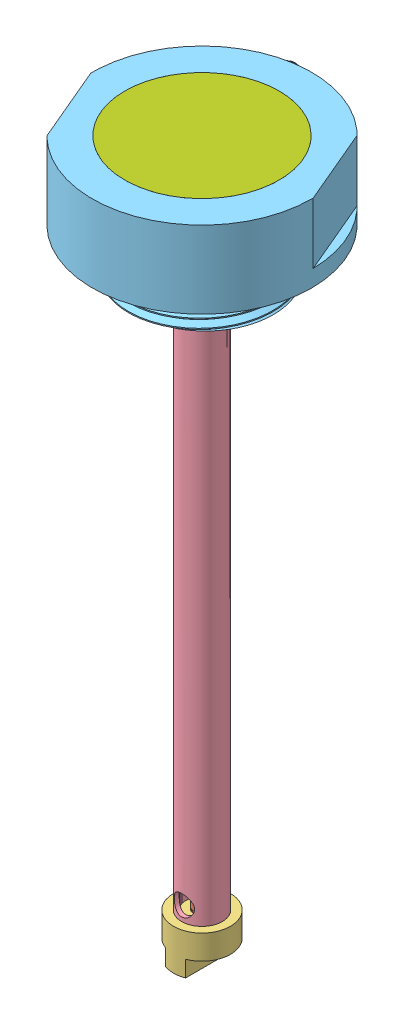
SolidWorks assembly assemblynew, configuration Default. Lengths in mm.
Overall size (70.81 175.04 84.92).
15 component instances, 12 part files, 30 mates.
Components (placement in the parent):
- top_insulator^assemblynew-1: top_insulator^assemblynew [Default] at origin size (21.03 11.69 20.56) (virtual)
- inner_rod^assemblynew-1: inner_rod^assemblynew [Default] at (0 0.457 0) x (0 0 1) z (-1 0 0) size (4.92 150.56 4.43) (virtual)
- bottom_insulator^assemblynew-1: bottom_insulator^assemblynew [Default] at (0 -145.036 0) size (14 10.25 14) (virtual)
- outer_tube^assemblynew-1: outer_tube^assemblynew [Default] at origin size (10 144.04 10) (virtual)
- outer_shell^assemblynew-1: outer_shell^assemblynew [Default] at (0 -10 0) x (-0.920505 0 0.390731) z (-0.390731 0 -0.920505) size (54 30.95 54) (virtual)
- PCB^assemblynew-1: PCB^assemblynew [Default] at (0 7 0) x (0.920505 0 -0.390731) z (0.390731 0 0.920505) size (34 3 22) (virtual)
- cap^assemblynew-1: cap^assemblynew [Default] at (0 15 0) size (40 5 40) (virtual)
- o-ring^assemblynew-1: o-ring^assemblynew [Default] at (0 1 0) size (44 2 44) (virtual)
- seal^assemblynew-1: seal^assemblynew [Default] at (0 10 0) x (0.920505 0 -0.390731) z (0.390731 0 0.920505) size (8 8 15.68) (virtual)
- cable^assemblynew-1: cable^assemblynew [Default] at (-6.2517 10 -14.7281) x (-0.920505 0 0.390731) z (-0.390731 0 -0.920505) size (11.12 53.19 43.28) (virtual)
- wires^assemblynew-1: wires^assemblynew [Default] at origin size (12.1 12.15 7.96) (virtual)
- screw^assemblynew-1: screw^assemblynew [Default] at (-9.7612 5 12.8343) size (4 4.47 4) (virtual)
- screw^assemblynew-2: screw^assemblynew [Default] at (-16.0129 5 -1.8938) size (4 4.47 4) (virtual)
- screw^assemblynew-3: screw^assemblynew [Default] at (16.0129 5 1.8938) x (0.694658 0 -0.71934) z (0.71934 0 0.694658) size (4 4.47 4) (virtual)
- screw^assemblynew-4: screw^assemblynew [Default] at (9.7612 5 -12.8343) x (0.694658 0 -0.71934) z (0.71934 0 0.694658) size (4 4.47 4) (virtual)
Mates (geometry in assembly coordinates):
- Coincident1: coordinate: point of ?
- Coincident2: coincident aligned: line of top_insulator^assemblynew-1 through (0 50.354 0) axis (0 -1 0); line of inner_rod^assemblynew-1 through (0 -19.5243 0) axis (0 -1 0)
- Coincident4: coincident aligned: plane of inner_rod^assemblynew-1 through (0 0.457 0) normal (0 0 1); plane of assembly through (0 0 0) normal (0 0 1)
- Distance1: distance = 0.457 mm aligned: plane of inner_rod^assemblynew-1 through (0 0.457 0) normal (0 1 0); plane of top_insulator^assemblynew-1 through (-1.6211 0 0) normal (0 1 0)
- Coincident5: coincident anti-aligned: line of inner_rod^assemblynew-1 through (0 -19.5243 0) axis (0 -1 0); line of bottom_insulator^assemblynew-1 through (0 -155.5486 0) axis (0 1 0)
- Coincident6: coincident aligned: plane of bottom_insulator^assemblynew-1 through (0 -145.036 0) normal (0 0 1); plane of assembly through (0 0 0) normal (0 0 1)
- Distance2: distance = 0.493 mm anti-aligned: plane of bottom_insulator^assemblynew-1 through (-1.6211 -150.036 0) normal (0 1 0); plane of inner_rod^assemblynew-1 through (0 -149.543 0) normal (0 -1 0)
- Coincident8: coordinate: unknown of ?
- Coincident9: coincident aligned: line of top_insulator^assemblynew-1 through (0 50.354 0) axis (0 -1 0); line of outer_shell^assemblynew-1 through (0 45 0) axis (0 -1 0)
- Coincident11: coincident anti-aligned: plane of top_insulator^assemblynew-1 through (-1.6211 0 0) normal (0 1 0); plane of outer_shell^assemblynew-1 through (7.9595 0 -3.3786) normal (0 -1 0)
- Angle1: planar angle = 2.740167 rad aligned: plane of outer_shell^assemblynew-1 through (0 -10 0) normal (-0.390731 0 -0.920505); plane of assembly through (0 0 0) normal (0 0 1)
- Coincident13: coincident anti-aligned: plane of outer_shell^assemblynew-1 through (-16.0129 7 -1.8938) normal (0 1 0); plane of PCB^assemblynew-1 through (9.2314 7 -11.523) normal (0 -1 0)
- Concentric1: concentric aligned: cylinder of outer_shell^assemblynew-1 through (-16.0129 7 -1.8938) axis (0 -1 0) radius 0.8647; cylinder of PCB^assemblynew-1 through (-16.0129 8 -1.8938) axis (0 -1 0) radius 1
- Concentric2: concentric aligned: cylinder of outer_shell^assemblynew-1 through (16.0129 7 1.8938) axis (0 -1 0) radius 0.8647; cylinder of PCB^assemblynew-1 through (16.0129 8 1.8938) axis (0 -1 0) radius 1
- Concentric3: concentric aligned: cylinder of outer_shell^assemblynew-1 through (0 5.0477 0) axis (0 1 0) radius 19; cylinder of cap^assemblynew-1 through (0 34.4438 0) axis (0 1 0) radius 19
- Coincident14: coincident aligned: plane of outer_shell^assemblynew-1 through (17.4896 20 -7.4239) normal (0 1 0); plane of cap^assemblynew-1 through (-19 20 0) normal (0 1 0)
- Coincident15: coincident aligned: plane of cap^assemblynew-1 through (0 15 0) normal (1 0 0); plane of assembly through (0 0 0) normal (1 0 0)
- Coincident16: coincident aligned: plane of o-ring^assemblynew-1 through (0 1 0) normal (1 0 0); plane of assembly through (0 0 0) normal (1 0 0)
- Coincident17: coincident aligned: plane of o-ring^assemblynew-1 through (0 1 0) normal (0 0 1); plane of assembly through (0 0 0) normal (0 0 1)
- Distance3: distance = 1 mm aligned: plane of o-ring^assemblynew-1 through (0 1 0) normal (0 1 0); plane of assembly through (0 0 0) normal (0 1 0)
- Concentric6: concentric aligned: cylinder of outer_shell^assemblynew-1 through (-10.5497 10 -24.8536) axis (0.390731 0 0.920505) radius 2.5; cylinder of seal^assemblynew-1 through (-12.8941 10 -30.3767) axis (0.390731 0 0.920505) radius 2.5
- Concentric7: concentric anti-aligned: cylinder of outer_shell^assemblynew-1 through (0 5.0477 0) axis (0 1 0) radius 19; cylinder of seal^assemblynew-1 through (0 15 0) axis (0 -1 0) radius 19
- Concentric8: concentric aligned: cylinder of seal^assemblynew-1 through (-12.8941 10 -30.3767) axis (0.390731 0 0.920505) radius 1.5; cylinder of cable^assemblynew-1 through (-12.8941 10 -30.3767) axis (0.390731 0 0.920505) radius 1.5
- Coincident19: coincident aligned: plane of seal^assemblynew-1 through (-12.8941 10 -30.3767) normal (-0.390731 0 -0.920505); circle of cable^assemblynew-1
- Perpendicular1: perpendicular: plane of cable^assemblynew-1 through (-6.2517 10 -14.7281) normal (-0.920505 0 0.390731); plane of assembly through (0 0 0) normal (0 1 0)
- Coincident20: coordinate: unknown of ?
- Concentric9: concentric anti-aligned: cylinder of PCB^assemblynew-1 through (-9.7612 8 12.8343) axis (0 -1 0) radius 1; cylinder of screw^assemblynew-1 through (-9.7612 17.4423 12.8343) axis (0 1 0) radius 1
- Coincident21: coincident anti-aligned: plane of PCB^assemblynew-1 through (9.2314 8 -11.523) normal (0 1 0); plane of screw^assemblynew-1 through (-8.7612 8 12.8343) normal (0 -1 0)
- Concentric10: concentric anti-aligned: cylinder of PCB^assemblynew-1 through (-16.0129 8 -1.8938) axis (0 -1 0) radius 1; cylinder of screw^assemblynew-2 through (-16.0129 17.4423 -1.8938) axis (0 1 0) radius 1
- Coincident22: coincident anti-aligned: plane of PCB^assemblynew-1 through (9.2314 8 -11.523) normal (0 1 0); plane of screw^assemblynew-2 through (-15.0129 8 -1.8938) normal (0 -1 0)
